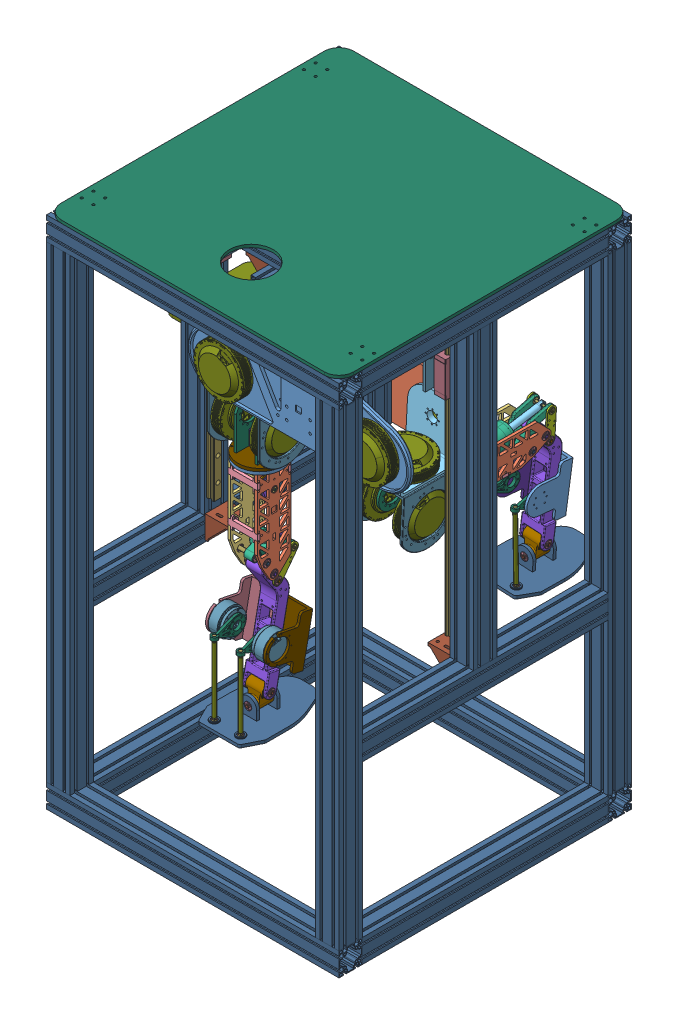
SolidWorks assembly 完整下肢, configuration 默认. Lengths in mm.
Overall size (1520 1770 1220).
259 component instances, 52 part files, 501 mates.
Components (placement in the parent):
- 髋一级连接板-1: 髋一级连接板 [默认] at (-1.8233 -129.1825 751.7525) size (760.75 280 18)
- 髋一级连接板_B-1: 髋一级连接板_B [默认] at (-1.8233 -129.1825 543.7525) size (760.75 280 18)
- 轴承_NSK635-1: 轴承_NSK635 [默认] at (238.0767 -238.3366 462.2655) x (0.049258 0.922114 0.38377) z (-0.020471 -0.383224 0.923429) size (19 6 19)
- 轴承_NSK635-2: 轴承_NSK635 [默认] at (-250.8233 -423.6825 652.2525) x (0 0.998125 -0.061201) z (0 0.061201 0.998125) size (19 6 19)
- 轴承_NSK635-3: 轴承_NSK635 [默认] at (142.2133 -233.2156 462.2655) x (0.049258 0.922114 0.38377) z (-0.020471 -0.383224 0.923429) size (19 6 19)
- 轴承_NSK635-4: 轴承_NSK635 [默认] at (-346.8233 -423.6825 652.2525) x (0 0.998125 -0.061201) z (0 0.061201 0.998125) size (19 6 19)
- 轴承_NSK6900NR-5: 轴承_NSK6900NR [默认] at (230.6224 -265.3994 255.8742) x (0.026574 0.497465 -0.867077) z (-0.046252 -0.865843 -0.498174) size (25 6 25)
- 轴承_NSK6900NR-6: 轴承_NSK6900NR [默认] at (231.9288 -240.9437 212.2827) x (0.026574 0.497465 -0.867077) z (-0.046252 -0.865843 -0.498174) size (25 6 25)
- 轴承_NSK6900NR-7: 轴承_NSK6900NR [默认] at (-256.8233 -630.3812 677.2525) x (0 0.205526 -0.978652) z (0 -0.978652 -0.205526) size (25 6 25)
- 轴承_NSK6900NR-8: 轴承_NSK6900NR [默认] at (140.7506 -260.5986 255.8742) x (0.049258 0.922114 0.38377) z (-0.020471 -0.383224 0.923429) size (25 6 25)
- 轴承_NSK6900NR-9: 轴承_NSK6900NR [默认] at (-256.8233 -673.6825 652.2525) x (0 0.205526 -0.978652) z (0 -0.978652 -0.205526) size (25 6 25)
- 轴承_NSK6900NR-10: 轴承_NSK6900NR [默认] at (-346.8233 -630.3812 677.2525) x (0 0.998125 -0.061201) z (0 0.061201 0.998125) size (25 6 25)
- 轴承_NSK6900NR-11: 轴承_NSK6900NR [默认] at (142.057 -236.1429 212.2827) x (0.049258 0.922114 0.38377) z (-0.020471 -0.383224 0.923429) size (25 6 25)
- 轴承_NSK6900NR-12: 轴承_NSK6900NR [默认] at (-346.8233 -673.6825 652.2525) x (0 0.998125 -0.061201) z (0 0.061201 0.998125) size (25 6 25)
- 轴承_NSK6900NR-17: 轴承_NSK6900NR [默认] at (176.6993 -262.5189 255.8742) x (0.000691 0.01293 0.999916) z (-0.053338 -0.998493 0.012949) size (25 6 25)
- 轴承_NSK6900NR-18: 轴承_NSK6900NR [默认] at (194.6737 -263.4791 255.8742) x (-0.021069 -0.394415 -0.918691) z (-0.049005 -0.917383 0.394978) size (25 6 25)
- 轴承_NSK6900NR-19: 轴承_NSK6900NR [默认] at (-310.8233 -630.3812 677.2525) x (0 -0.990009 -0.141004) z (0 0.141004 -0.990009) size (25 6 25)
- 轴承_NSK6900NR-20: 轴承_NSK6900NR [默认] at (-292.8233 -630.3812 677.2525) x (0 0.96851 -0.248973) z (0 -0.248973 -0.96851) size (25 6 25)
- 轴承_NSK6900NR-37: 轴承_NSK6900NR [默认] at (-324.8233 -1030.6139 652.2525) x (0 -0.237164 0.97147) z (0 -0.97147 -0.237164) size (25 6 25)
- 轴承_NSK6900NR-38: 轴承_NSK6900NR [默认] at (-278.8233 -1030.6139 652.2525) x (0 -0.153045 -0.988219) z (0 -0.988219 0.153045) size (25 6 25)
- 轴承_NSK6900NR-39: 轴承_NSK6900NR [默认] at (-301.8233 -1070.6139 629.2525) x (0.998149 0.060814 0) z (-0.060814 0.998149 0) size (25 6 25)
- 轴承_NSK6900NR-40: 轴承_NSK6900NR [默认] at (-301.8233 -1070.6139 675.2525) x (-0.802358 -0.596843 0) z (-0.596843 0.802358 0) size (25 6 25)
- 轴承_NSK6900NR-41: 轴承_NSK6900NR [默认] at (165.9394 -632.6645 198.3743) x (0.811883 -0.583783 0.006592) z (-0.58382 -0.811818 0.010283) size (25 6 25)
- 轴承_NSK6900NR-42: 轴承_NSK6900NR [默认] at (191.0252 -594.2319 174.8875) x (0.018298 0.342539 0.939325) z (0.050106 0.937988 -0.343027) size (25 6 25)
- 轴承_NSK6900NR-43: 轴承_NSK6900NR [默认] at (145.0907 -591.7781 174.8875) x (-0.004431 -0.082951 0.996544) z (-0.053158 -0.995125 -0.083069) size (25 6 25)
- 轴承_NSK6900NR-44: 轴承_NSK6900NR [默认] at (165.9094 -633.2256 152.3778) x (-0.360366 0.932744 -0.011143) z (-0.932811 -0.360332 0.005003) size (25 6 25)
- 轴承_NSK6900NR-45: 轴承_NSK6900NR [默认] at (-301.8233 -1070.6139 687.2525) x (-0.919919 -0.392109 0) z (-0.392109 0.919919 0) size (25 6 25)
- 轴承_NSK6900NR-46: 轴承_NSK6900NR [默认] at (-301.8233 -1070.6139 617.2525) x (0.999952 0.009828 0) z (-0.009828 0.999952 0) size (25 6 25)
- 轴承_NSK6900NR-47: 轴承_NSK6900NR [默认] at (165.9472 -632.5182 210.3734) x (-0.999254 0.038618 0.00018) z (0.038613 0.99918 -0.012213) size (25 6 25)
- 轴承_NSK6900NR-48: 轴承_NSK6900NR [默认] at (165.9016 -633.3719 140.3787) x (0.908248 -0.418407 0.004512) z (0.418431 0.908178 -0.01135) size (25 6 25)
- 轴承_NSK6900NR-33: 轴承_NSK6900NR [默认] at (-336.8233 -1030.6139 652.2525) x (0 -0.947209 0.320618) z (0 -0.320618 -0.947209) size (25 6 25)
- 轴承_NSK6900NR-34: 轴承_NSK6900NR [默认] at (203.0082 -594.872 174.8875) x (-0.049795 -0.932169 0.358581) z (0.019128 0.358071 0.933498) size (25 6 25)
- 轴承_NSK6900NR-35: 轴承_NSK6900NR [默认] at (-266.8233 -1030.6139 652.2525) x (0 -0.998208 -0.059843) z (0 -0.059843 0.998208) size (25 6 25)
- 轴承_NSK6900NR-36: 轴承_NSK6900NR [默认] at (133.1078 -591.138 174.8875) x (-0.053286 -0.997519 -0.046007) z (0.002454 0.045942 -0.998941) size (25 6 25)
- 轴承_NSK635-6: 轴承_NSK635 [默认] at (-275.8233 -643.2766 570.5287) x (0 0.998125 -0.061201) z (0 0.061201 0.998125) size (19 6 19)
- 轴承_NSK635-7: 轴承_NSK635 [默认] at (215.7047 -188.4726 179.8677) x (0.049258 0.922114 0.38377) z (-0.020471 -0.383224 0.923429) size (19 6 19)
- 轴承_NSK635-8: 轴承_NSK635 [默认] at (-321.8233 -643.2766 570.5287) x (0 0.998125 -0.061201) z (0 0.061201 0.998125) size (19 6 19)
- 轴承_NSK635-9: 轴承_NSK635 [默认] at (169.7702 -186.0189 179.8677) x (0.049258 0.922114 0.38377) z (-0.020471 -0.383224 0.923429) size (19 6 19)
- 轴承_NSK6900NR-21: 轴承_NSK6900NR [默认] at (215.8968 -278.61 180.3417) x (0.026574 0.497465 -0.867077) z (-0.046252 -0.865843 -0.498174) size (25 6 25)
- 轴承_NSK6900NR-22: 轴承_NSK6900NR [默认] at (153.9851 -275.3027 180.3417) x (0.047078 0.8813 0.470205) z (-0.025082 -0.469536 0.882557) size (25 6 25)
- 轴承_NSK6900NR-23: 轴承_NSK6900NR [默认] at (-332.8233 -715.285 624.5175) x (0 0.998125 -0.061201) z (0 0.061201 0.998125) size (25 6 25)
- 轴承_NSK6900NR-24: 轴承_NSK6900NR [默认] at (-270.8233 -715.285 624.5175) x (0 0.205526 -0.978652) z (0 -0.978652 -0.205526) size (25 6 25)
- 轴承_NSK6900NR-25: 轴承_NSK6900NR [默认] at (163.0271 -237.2631 212.2827) x (-0.000432 -0.00809 0.999967) z (-0.053341 -0.998543 -0.008101) size (25 6 25)
- 轴承_NSK6900NR-26: 轴承_NSK6900NR [默认] at (210.9587 -239.8235 212.2827) x (-0.022004 -0.411917 -0.910956) z (-0.048593 -0.909659 0.412504) size (25 6 25)
- 轴承_NSK6900NR-27: 轴承_NSK6900NR [默认] at (160.9751 -275.6761 180.3417) x (-0.000432 -0.00809 0.999967) z (-0.053341 -0.998543 -0.008101) size (25 6 25)
- 轴承_NSK6900NR-28: 轴承_NSK6900NR [默认] at (208.9068 -278.2366 180.3417) x (-0.000432 -0.00809 0.999967) z (0.053341 0.998543 0.008101) size (25 6 25)
- 轴承_NSK6900NR-29: 轴承_NSK6900NR [默认] at (-325.8233 -673.6825 652.2525) x (0 -0.98581 -0.167864) z (0 0.167864 -0.98581) size (25 6 25)
- 轴承_NSK6900NR-30: 轴承_NSK6900NR [默认] at (-277.8233 -715.285 624.5175) x (0 -0.98581 -0.167864) z (0 -0.167864 0.98581) size (25 6 25)
- 轴承_NSK6900NR-31: 轴承_NSK6900NR [默认] at (-325.8233 -715.285 624.5175) x (0 0.974921 -0.222553) z (0 0.222553 0.974921) size (25 6 25)
- 轴承_NSK6900NR-32: 轴承_NSK6900NR [默认] at (-277.8233 -673.6825 652.2525) x (0 0.974921 -0.222553) z (0 -0.222553 -0.974921) size (25 6 25)
- 轴承_NSK635-10: 轴承_NSK635 [默认] at (-270.8233 -643.2766 570.5287) x (0 0.138285 -0.990392) z (0 -0.990392 -0.138285) size (19 6 19)
- 轴承_NSK635-11: 轴承_NSK635 [默认] at (158.7858 -185.4321 179.8677) x (0.000691 0.01293 0.999916) z (-0.053338 -0.998493 0.012949) size (19 6 19)
- 轴承_NSK635-12: 轴承_NSK635 [默认] at (-338.8233 -643.2766 570.5287) x (0 0.091476 -0.995807) z (0 -0.995807 -0.091476) size (19 6 19)
- 轴承_NSK635-13: 轴承_NSK635 [默认] at (226.689 -189.0594 179.8677) x (0.000691 0.01293 0.999916) z (-0.053338 -0.998493 0.012949) size (19 6 19)
- 髋二级连接板_旋转-1: 髋二级连接板_旋转 [默认] at (-216.8233 -124.1825 562.2525) x (0 0 -1) z (-1 0 0) size (206.5 183 170)
- 髋二级连接板_旋转-2: 髋二级连接板_旋转 [默认] at (277.9881 -128.5814 562.2525) x (0 0 -1) z (-0.998576 0.053343 0) size (206.5 183 170)
- 大腿_电机轴-1: 大腿_电机轴 [默认] at (241.0724 -238.4966 462.2655) x (0.049258 0.922114 0.38377) z (-0.020471 -0.383224 0.923429) size (5 108 5)
- 大腿_电机轴-2: 大腿_电机轴 [默认] at (-247.8233 -423.6825 652.2525) x (0 -0.967053 0.254576) z (0 -0.254576 -0.967053) size (5 108 5)
- 上下连杆轴-1: 上下连杆轴 [默认] at (229.6848 -189.2194 179.8677) x (-0.049961 -0.935279 -0.350368) z (-0.998576 0.053343 0) size (5 5 80)
- 上下连杆轴-2: 上下连杆轴 [默认] at (-341.8233 -643.2766 570.5287) x (0 0.004287 -0.999991) z (1 0 0) size (5 5 80)
- 大腿小腿轴-1: 大腿小腿轴 [默认] at (186.9929 -238.5433 212.2827) x (0.050119 0.93823 0.342364) z (-0.018263 -0.341876 0.939568) size (10 108 10)
- 大腿小腿轴-2: 大腿小腿轴 [默认] at (-301.8233 -673.6825 652.2525) x (0 0.99823 -0.059474) z (0 0.059474 0.99823) size (10 108 10)
- 下连杆小腿轴-1: 下连杆小腿轴 [默认] at (184.9409 -276.9563 180.3417) x (0.049345 0.923729 0.379855) z (-0.020263 -0.379314 0.925046) size (10 80 10)
- 下连杆小腿轴-2: 下连杆小腿轴 [默认] at (-301.8233 -715.285 624.5175) x (0 0.99823 -0.059474) z (0 0.059474 0.99823) size (10 80 10)
- 上连杆大腿轴-1: 上连杆大腿轴 [默认] at (-301.8233 -630.3812 677.2525) x (0 0.998125 -0.061201) z (0 0.061201 0.998125) size (10 108 10)
- 上连杆大腿轴-2: 上连杆大腿轴 [默认] at (185.6865 -262.999 255.8742) x (0.049258 0.922114 0.38377) z (-0.020471 -0.383224 0.923429) size (10 108 10)
- 踝关节轴-3: 踝关节轴 [默认] at (-301.8233 -1070.6139 652.2525) x (0.999952 0.009828 0) z (-0.009828 0.999952 0) size (10 88 10)
- 踝关节轴-4: 踝关节轴 [默认] at (165.9244 -632.945 175.376) x (0.908248 -0.418407 0.004512) z (0.418431 0.908178 -0.01135) size (10 88 10)
- 踝关节轴-1: 踝关节轴 [默认] at (168.058 -593.005 174.8875) x (-0.048986 -0.917023 0.395815) z (0.021114 0.395252 0.91833) size (10 88 10)
- 踝关节轴-2: 踝关节轴 [默认] at (-301.8233 -1030.6139 652.2525) x (0 -0.998208 -0.059843) z (0 -0.059843 0.998208) size (10 88 10)
- 轴套-3: 轴套 [d5L40.5大腿板与电机] at (182.6557 -235.376 462.2655) x (0.000691 0.01293 0.999916) z (-0.998576 0.053343 0) size (7 7 40.5)
- 轴套-4: 轴套 [d5L40.5大腿板与电机] at (232.0852 -238.0165 462.2655) x (0.000691 0.01293 0.999916) z (-0.998576 0.053343 0) size (7 7 40.5)
- 轴套-5: 轴套 [d5L40.5大腿板与电机] at (-297.3233 -423.6825 652.2525) x (0 0.004287 -0.999991) z (1 0 0) size (7 7 40.5)
- 轴套-6: 轴套 [d5L40.5大腿板与电机] at (-346.8233 -423.6825 652.2525) x (0 0.004287 -0.999991) z (1 0 0) size (7 7 40.5)
- 轴套-11: 轴套 [d5L5上下连杆] at (-332.8233 -643.2766 570.5287) x (0 0.259292 -0.965799) z (1 0 0) size (7 7 5)
- 轴套-12: 轴套 [d5L5上下连杆] at (163.7787 -185.6988 179.8677) x (0.000691 0.01293 0.999916) z (-0.998576 0.053343 0) size (7 7 5)
- 轴套-13: 轴套 [d5L5上下连杆] at (-275.8233 -643.2766 570.5287) x (0 0.004287 -0.999991) z (1 0 0) size (7 7 5)
- 轴套-14: 轴套 [d5L5上下连杆] at (220.6976 -188.7394 179.8677) x (0.000691 0.01293 0.999916) z (-0.998576 0.053343 0) size (7 7 5)
- 轴套-15: 轴套 [d5L15.5上连杆与推杆] at (209.7132 -188.1526 179.8677) x (0.000691 0.01293 0.999916) z (-0.998576 0.053343 0) size (7 7 15.5)
- 轴套-16: 轴套 [d5L15.5上连杆与推杆] at (185.2481 -186.8457 179.8677) x (0.007725 0.144605 0.989459) z (-0.998576 0.053343 0) size (7 7 15.5)
- 轴套-17: 轴套 [d5L15.5上连杆与推杆] at (-297.3233 -643.2766 570.5287) x (0 0.004287 -0.999991) z (1 0 0) size (7 7 15.5)
- 轴套-18: 轴套 [d5L15.5上连杆与推杆] at (-321.8233 -643.2766 570.5287) x (0 0.004287 -0.999991) z (1 0 0) size (7 7 15.5)
- 轴套-19: 轴套 [d10L15大小腿] at (231.9288 -240.9437 212.2827) x (0.00702 0.131424 0.991301) z (-0.998576 0.053343 0) size (12 12 15)
- 轴套-20: 轴套 [d10L15大小腿] at (-346.8233 -673.6825 652.2525) x (0 0.00111 -0.999999) z (1 0 0) size (12 12 15)
- 轴套-21: 轴套 [d10L15大小腿] at (157.0356 -236.943 212.2827) x (-0.000432 -0.00809 0.999967) z (-0.998576 0.053343 0) size (12 12 15)
- 轴套-22: 轴套 [d10L15大小腿] at (-271.8233 -673.6825 652.2525) x (0 -0.961131 -0.276091) z (1 0 0) size (12 12 15)
- 轴套-23: 轴套 [d10L1小腿下连杆] at (-331.8233 -715.285 624.5175) x (0 0.98581 0.167864) z (-1 0 0) size (12 12 1)
- 轴套-24: 轴套 [d10L1小腿下连杆] at (153.9851 -275.3027 180.3417) x (-0.029978 -0.561194 -0.827141) z (0.998576 -0.053343 0) size (12 12 1)
- 轴套-25: 轴套 [d10L1小腿下连杆] at (-271.8233 -715.285 624.5175) x (0 0.011403 -0.999935) z (1 0 0) size (12 12 1)
- 轴套-26: 轴套 [d10L1小腿下连杆] at (215.8968 -278.61 180.3417) x (-0.000432 -0.00809 0.999967) z (-0.998576 0.053343 0) size (12 12 1)
- 轴套-7: 轴套 [d10L30大腿上连杆] at (170.7079 -262.1989 255.8742) x (-0.024462 -0.457931 0.888651) z (-0.998576 0.053343 0) size (12 12 30)
- 轴套-8: 轴套 [d10L30大腿上连杆] at (230.6224 -265.3994 255.8742) x (0.001085 0.020314 0.999793) z (-0.998576 0.053343 0) size (12 12 30)
- 轴套-9: 轴套 [d10L30大腿上连杆] at (-286.8233 -630.3812 677.2525) x (0 0.004287 -0.999991) z (1 0 0) size (12 12 30)
- 轴套-10: 轴套 [d10L30大腿上连杆] at (-346.8233 -630.3812 677.2525) x (0 -0.022464 -0.999748) z (1 0 0) size (12 12 30)
- 轴套V2-1: 轴套V2 [d10L6踝关节] at (-272.8233 -1030.6139 652.2525) x (0 0.885448 0.464738) z (1 0 0) size (12 12 6)
- 轴套V2-2: 轴套V2 [d10L6踝关节] at (-336.8233 -1030.6139 652.2525) x (0 -0.178991 -0.983851) z (1 0 0) size (12 12 6)
- 轴套V2-3: 轴套V2 [d10L6踝关节] at (139.0993 -591.458 174.8875) x (-0.003743 -0.070062 0.997536) z (-0.998576 0.053343 0) size (12 12 6)
- 轴套V2-4: 轴套V2 [d10L6踝关节] at (203.0082 -594.872 174.8875) x (-0.012193 -0.228259 0.973524) z (-0.998576 0.053343 0) size (12 12 6)
- 轴套-27: 轴套 [d10L6踝关节] at (-301.8233 -1070.6139 681.2525) x (0.999952 0.009828 0) z (0 0 1) size (12 12 6)
- 轴套-28: 轴套 [d10L6踝关节] at (-301.8233 -1070.6139 617.2525) x (0.999952 0.009828 0) z (0 0 1) size (12 12 6)
- 轴套-29: 轴套 [d10L6踝关节] at (165.9016 -633.3719 140.3787) x (0.908248 -0.418407 0.004512) z (0.000652 0.012197 0.999925) size (12 12 6)
- 轴套-30: 轴套 [d10L6踝关节] at (165.9433 -632.5913 204.3739) x (0.908248 -0.418407 0.004512) z (0.000652 0.012197 0.999925) size (12 12 6)
- 髋三级连接板_前摆V2-1: 髋三级连接板_前摆V2 [默认] at (181.9338 -333.249 562.2525) x (0.998576 -0.053343 0) z (0 0 1) size (180 200 180)
- 髋三级连接板_前摆V2-2: 髋三级连接板_前摆V2 [默认] at (-301.8233 -333.6825 742.2525) x (-1 0 0) z (0 0 -1) size (180 200 180)
- 腿髋转接架侧板V2-1: 腿髋转接架侧板V2 [默认] at (227.1486 -236.696 552.2594) x (-0.053339 -0.998508 0.011726) z (-0.998576 0.053343 0) size (96 150 8)
- 腿髋转接架侧板V2-2: 腿髋转接架侧板V2 [默认] at (147.2625 -232.4286 552.2594) x (0.053339 0.998508 -0.011726) z (0.998576 -0.053343 0) size (96 150 8)
- 腿髋转接架侧板V2-3: 腿髋转接架侧板V2 [默认] at (-261.8233 -333.6825 652.2525) x (0 0 1) z (-1 0 0) size (96 150 8)
- 腿髋转接架侧板V2-4: 腿髋转接架侧板V2 [默认] at (-341.8233 -333.6825 652.2525) x (0 0 -1) z (1 0 0) size (96 150 8)
- B1电机模型-1: B1电机模型 [默认] at (349.6629 49.3918 700.037) x (0 0 1) z (-0.906308 -0.422618 0) size (57.67 170.5 170.5)
- B1电机模型-2: B1电机模型 [默认] at (181.2585 -154.384 500.7663) x (0.998576 -0.053343 0) z (-0.022544 -0.422017 0.906308) size (57.67 170.5 170.5)
- B1电机模型-3: B1电机模型 [默认] at (193.9731 -299.3815 809.8173) x (-0.998576 0.053343 0) z (0.022544 0.422017 -0.906308) size (57.67 170.5 170.5)
- B1电机模型-4: B1电机模型 [默认] at (-144.2585 -94.7211 700.037) x (0 0 1) z (-0.906308 0.422618 0) size (57.67 170.5 170.5)
- B1电机模型-6: B1电机模型 [默认] at (124.4785 -180.1818 809.8173) x (0.053343 0.998576 0) z (0.422017 -0.022544 -0.906308) size (57.67 170.5 170.5)
- B1电机模型-7: B1电机模型 [默认] at (-380.3976 -183.898 500.7663) x (0 1 0) z (0.422618 0 0.906308) size (57.67 170.5 170.5)
- B1电机模型-10: B1电机模型 [默认] at (-291.6078 -299.2211 809.8173) x (-1 0 0) z (0 0.422618 -0.906308) size (57.67 170.5 170.5)
- B1电机模型-11: B1电机模型 [默认] at (-312.0388 -155.1082 500.7663) x (1 0 0) z (0 -0.422618 0.906308) size (57.67 170.5 170.5)
- 腿髋转接架连接板V2-1: 腿髋转接架连接板V2 [默认] at (-333.8233 -333.6825 647.2525) size (30 50 10)
- 腿髋转接架连接板V2-2: 腿髋转接架连接板V2 [默认] at (218.8933 -241.2618 552.318) x (-0.998576 0.053343 0) z (0.053339 0.998508 -0.011726) size (30 50 10)
- 腿髋转接架连接板V2-3: 腿髋转接架连接板V2 [默认] at (155.5178 -227.8628 552.2007) x (0.998576 -0.053343 0) z (-0.053339 -0.998508 0.011726) size (30 50 10)
- 腿髋转接架连接板V2-4: 腿髋转接架连接板V2 [默认] at (-269.8233 -333.6825 657.2525) x (-1 0 0) z (0 0 -1) size (30 50 10)
- 腿髋转接架底座V2-1: 腿髋转接架底座V2 [默认] at (187.2056 -234.5623 552.2594) x (-0.998576 0.053343 0) z (-0.053339 -0.998508 0.011726) size (150 10 150)
- 腿髋转接架底座V2-2: 腿髋转接架底座V2 [默认] at (-301.8233 -333.6825 652.2525) x (-1 0 0) z (0 0 1) size (150 10 150)
- 大腿主干_上板V2-1: 大腿主干_上板V2 [默认] at (-301.8233 -673.6825 602.2525) size (150 10 150)
- 大腿主干_上板V2-2: 大腿主干_上板V2 [默认] at (189.6599 -188.6179 211.6964) x (0.998576 -0.053343 0) z (-0.053339 -0.998508 0.011726) size (150 10 150)
- 大腿主干_右侧板V2-1: 大腿主干_右侧板V2 [默认] at (236.9217 -241.2105 212.2827) x (-0.053339 -0.998508 0.011726) z (-0.998576 0.053343 0) size (116 518 200.95)
- 大腿主干_右侧板V2-2: 大腿主干_右侧板V2 [默认] at (-251.8233 -673.6825 652.2525) x (0 0 1) z (-1 0 0) size (116 518 200.95)
- 大腿主干_左侧板V2-1: 大腿主干_左侧板V2 [默认] at (236.9217 -241.2105 212.2827) x (-0.053339 -0.998508 0.011726) z (-0.998576 0.053343 0) size (116 518 200.95)
- 大腿主干_左侧板V2-2: 大腿主干_左侧板V2 [默认] at (-251.8233 -673.6825 652.2525) x (0 0 1) z (-1 0 0) size (116 518 200.95)
- 大腿侧板连接V2-1: 大腿侧板连接V2 [默认] at (233.9061 -297.6638 337.6571) x (0.000625 0.011709 0.999931) z (-0.998576 0.053343 0) size (40 20 100)
- 大腿侧板连接V2-2: 大腿侧板连接V2 [默认] at (-351.8233 -398.6825 594.2525) x (0 1 0) z (1 0 0) size (40 20 100)
- 大腿侧板连接V2-3: 大腿侧板连接V2 [默认] at (-251.8233 -548.9797 710.2525) x (0 1 0) z (-1 0 0) size (40 20 100)
- 大腿侧板连接V2-4: 大腿侧板连接V2 [默认] at (234.0001 -295.9039 487.9439) x (0.000625 0.011709 0.999931) z (-0.998576 0.053343 0) size (40 20 100)
- 大腿侧板连接V2-5: 大腿侧板连接V2 [默认] at (240.1999 -179.8429 506.5824) x (-0.000625 -0.011709 -0.999931) z (-0.998576 0.053343 0) size (40 20 100)
- 大腿侧板连接V2-6: 大腿侧板连接V2 [默认] at (-251.8233 -398.6825 710.2525) x (0 1 0) z (-1 0 0) size (40 20 100)
- 大腿主干_连接块-1: 大腿主干_连接块 [默认] at (228.4014 -231.991 532.2021) x (-0.998576 0.053343 0) z (-0.053339 -0.998508 0.011726) size (40 50 10)
- 大腿主干_连接块-2: 大腿主干_连接块 [默认] at (145.9847 -237.6019 532.3194) x (0.998576 -0.053343 0) z (0.053339 0.998508 -0.011726) size (40 50 10)
- 大腿主干_连接块-3: 大腿主干_连接块 [默认] at (-342.8233 -353.6825 657.2525) x (1 0 0) z (0 0 -1) size (40 50 10)
- 大腿主干_连接块-4: 大腿主干_连接块 [默认] at (-260.8233 -353.6825 647.2525) x (-1 0 0) z (0 0 1) size (40 50 10)
- 膝盖上连杆_107.5V2-1: 膝盖上连杆_107.5V2 [默认] at (224.6919 -188.9527 179.8677) x (-0.051524 -0.964525 -0.258915) z (-0.998576 0.053343 0) size (83.75 123.1 70)
- 膝盖上连杆_107.5V2-2: 膝盖上连杆_107.5V2 [默认] at (-266.8233 -643.2766 570.5287) x (0 -0.799794 0.600275) z (-1 0 0) size (83.75 123.1 70)
- 膝关节下连杆_90-1: 膝关节下连杆_90 [默认] at (220.8897 -278.8767 180.3417) x (0.000281 0.005259 0.999986) z (-0.998576 0.053343 0) size (30 120 76)
- 膝关节下连杆_90-2: 膝关节下连杆_90 [默认] at (-337.8233 -715.285 624.5175) x (0 -0.599875 -0.800094) z (1 0 0) size (30 120 76)
- 小腿主干-1: 小腿主干 [默认] at (216.9502 -240.1436 212.2827) x (0.004924 0.092171 0.995731) z (-0.998576 0.053343 0) size (110 390 143.66)
- 小腿主干-2: 小腿主干 [默认] at (-271.8233 -673.6825 652.2525) x (0 0.196116 0.980581) z (-1 0 0) size (110 390 143.66)
- 脚踝十字连接-1: 脚踝十字连接 [默认] at (-330.8233 -1030.6139 652.2525) x (0 -1 0) z (1 0 0) size (80 58 58)
- 脚踝十字连接-2: 脚踝十字连接 [默认] at (197.0167 -594.5519 174.8875) x (-0.053339 -0.998502 0.012214) z (-0.998576 0.053343 0) size (80 58 58)
- 球铰脚底板-1: 球铰脚底板 [默认] at (-301.8233 -1110.6139 792.2525) size (200 93.12 300)
- 球铰脚底板-2: 球铰脚底板 [默认] at (163.8821 -671.1776 315.8542) x (0.998576 -0.053343 0) z (0.000652 0.012197 0.999925) size (200 93.12 300)
- 关节轴承外圈_SQD6-1: 关节轴承外圈_SQD6 [默认] at (209.1919 -666.5799 285.7663) x (-0.053339 -0.998502 0.012214) z (0.009299 0.011734 0.999888) size (6.75 18 18)
- 关节轴承外圈_SQD6-2: 关节轴承外圈_SQD6 [默认] at (119.32 -661.7791 285.7663) x (-0.053339 -0.998502 0.012214) z (0.009299 0.011734 0.999888) size (6.75 18 18)
- 关节轴承外圈_SQD6-3: 关节轴承外圈_SQD6 [默认] at (-256.8233 -1103.2389 762.2525) x (0 -1 0) z (-0.68418 0 0.729313) size (6.75 18 18)
- 关节轴承外圈_SQD6-4: 关节轴承外圈_SQD6 [默认] at (-346.8233 -1103.2389 762.2525) x (0 -1 0) z (-0.68418 0 0.729313) size (6.75 18 18)
- 关节轴承内杆_SQD6-1: 关节轴承内杆_SQD6 [默认] at (-346.8233 -1103.2389 762.2525) x (0.998471 0 -0.055281) z (0.055281 0.000001 0.998471) size (14 37.17 14)
- 关节轴承内杆_SQD6-2: 关节轴承内杆_SQD6 [默认] at (-256.8233 -1103.2389 762.2525) x (0.998075 0 -0.062014) z (0.062014 0.000001 0.998075) size (14 37.17 14)
- 关节轴承内杆_SQD6-3: 关节轴承内杆_SQD6 [默认] at (119.32 -661.7791 285.7663) x (0.707856 -0.086337 0.70106) z (-0.704349 -0.011501 0.70976) size (14 37.17 14)
- 关节轴承内杆_SQD6-4: 关节轴承内杆_SQD6 [默认] at (209.1919 -666.5799 285.7663) x (0.998399 -0.051754 -0.02282) z (0.019165 -0.070057 0.997359) size (14 37.17 14)
- 小腿左侧电机安装板A1-1: 小腿左侧电机安装板A1 [默认] at (-404.8233 -957.0654 606.9487) x (1 0 0) z (0 0.196116 0.980581) size (99.5 170 146)
- A1电机-1: A1电机 [默认] at (-395.8233 -854.1044 688.3369) x (0 0.194064 -0.980989) z (1 0 0) size (92 92 49)
- 小腿电机摇杆A1-1: 小腿电机摇杆A1 [默认] at (-343.8233 -854.1044 688.3369) x (0 0.002916 0.999996) z (-1 0 0) size (114.92 60 22)
- 关节轴承外圈_SQD6-5: 关节轴承外圈_SQD6 [默认] at (-346.8233 -853.8889 762.2522) x (0 -0.999996 0.002916) z (0.078101 0.002907 0.996941) size (6.75 18 18)
- 关节轴承内杆_SQD6-5: 关节轴承内杆_SQD6 [默认] at (-346.8233 -853.8889 762.2522) x (-0.959854 0 -0.280502) z (-0.280502 0.000001 0.959854) size (14 37.17 14)
- 踝关节连杆-1: 踝关节连杆 [默认] at (-346.8233 -1091.0639 762.2525) x (0.267051 -0.000001 -0.963682) z (0 1 -0.000001) size (12 12 225)
- 小腿左侧定脚踝安装板-1: 小腿左侧定脚踝安装板 [默认] at (114.2954 -512.1318 137.5386) x (0.998576 -0.053343 0) z (0.004924 0.092171 0.995731) size (54.5 170 146)
- 小腿电机摇杆A1-3: 小腿电机摇杆A1 [默认] at (135.2798 -419.2516 229.2659) x (0.00413 0.077315 0.996998) z (-0.998576 0.053343 0) size (114.92 60 22)
- 关节轴承内杆_SQD6-6: 关节轴承内杆_SQD6 [默认] at (132.5894 -413.3767 302.9597) x (0.23447 -0.079585 0.96886) z (0.970666 -0.035391 -0.237814) size (14 37.17 14)
- 关节轴承外圈_SQD6-6: 关节轴承外圈_SQD6 [默认] at (132.5894 -413.3767 302.9597) x (0.053183 0.995579 -0.077426) z (-0.981979 0.066222 0.177009) size (6.75 18 18)
- 踝关节连杆-2: 踝关节连杆 [默认] at (131.9415 -425.5054 302.1202) x (-0.140449 -0.060897 0.988213) z (-0.053216 -0.9962 -0.068953) size (12 12 225)
- 镜向小腿左侧电机安装板A1-3: 镜向小腿左侧电机安装板A1 [默认] at (-198.8233 -957.0654 606.9487) x (-1 0 0) z (0 -0.196116 -0.980581) size (99.5 170 146)
- 镜向小腿左侧定脚踝安装板-2: 镜向小腿左侧定脚踝安装板 [默认] at (230.1303 -518.3196 137.5386) x (-0.998576 0.053343 0) z (-0.004924 -0.092171 -0.995731) size (54.5 170 146)
- 小腿电机摇杆A1-4: 小腿电机摇杆A1 [默认] at (225.1517 -424.0524 229.2659) x (0.00413 0.077315 0.996998) z (-0.998576 0.053343 0) size (114.92 60 22)
- 关节轴承内杆_SQD6-8: 关节轴承内杆_SQD6 [默认] at (222.4612 -418.1776 302.9597) x (0.994388 -0.059188 0.087687) z (0.091435 0.063899 -0.993759) size (14 37.17 14)
- 关节轴承外圈_SQD6-8: 关节轴承外圈_SQD6 [默认] at (222.4612 -418.1776 302.9597) x (0.053183 0.995579 -0.077426) z (-0.112914 0.083033 0.990129) size (6.75 18 18)
- 踝关节连杆-4: 踝关节连杆 [默认] at (209.8398 -654.4512 286.6058) x (0.99813 -0.055144 0.026366) z (0.053216 0.9962 0.068953) size (12 12 225)
- 小腿电机摇杆A1-5: 小腿电机摇杆A1 [默认] at (-253.8233 -854.1044 688.3369) x (0 0.002916 0.999996) z (-1 0 0) size (114.92 60 22)
- A1电机-3: A1电机 [默认] at (-207.8233 -854.1044 688.3369) x (0 -0.194064 0.980989) z (-1 0 0) size (92 92 49)
- 关节轴承内杆_SQD6-9: 关节轴承内杆_SQD6 [默认] at (-256.8233 -853.8889 762.2522) x (0.971204 0 -0.238248) z (-0.238248 -0.000001 -0.971204) size (14 37.17 14)
- 关节轴承外圈_SQD6-9: 关节轴承外圈_SQD6 [默认] at (-256.8233 -853.8889 762.2522) x (0 -0.999996 0.002916) z (-0.243757 0.002828 0.969832) size (6.75 18 18)
- 踝关节连杆-5: 踝关节连杆 [默认] at (-256.8233 -866.0639 762.2522) x (0.999941 0 -0.010841) z (0 -1 0.000001) size (12 12 225)
- 轴用挡圈GB894-5-1: 轴用挡圈GB894-5 [默认] at (135.7226 -232.8689 462.2655) x (-0.050634 -0.947874 0.314595) z (0.016781 0.314148 0.949226) size (6.4 0.5 7.57)
- 轴用挡圈GB894-5-2: 轴用挡圈GB894-5 [默认] at (-352.8233 -423.6825 652.2525) x (0 0.998504 -0.054676) z (0 0.054676 0.998504) size (6.4 0.5 7.57)
- 轴用挡圈GB894-5-3: 轴用挡圈GB894-5 [默认] at (-250.3233 -423.6825 652.2525) x (0 0.998504 -0.054676) z (0 0.054676 0.998504) size (6.4 0.5 7.57)
- 轴用挡圈GB894-5-4: 轴用挡圈GB894-5 [默认] at (238.576 -238.3632 462.2655) x (-0.052938 -0.991004 0.122918) z (-0.006557 -0.122743 -0.992417) size (6.4 0.5 7.57)
- 轴用挡圈GB894-5-5: 轴用挡圈GB894-5 [默认] at (-264.3233 -643.2766 570.5287) x (0 0.998504 -0.054676) z (0 0.054676 0.998504) size (6.4 0.5 7.57)
- 轴用挡圈GB894-5-6: 轴用挡圈GB894-5 [默认] at (227.1883 -189.0861 179.8677) x (-0.052938 -0.991004 0.122918) z (-0.006557 -0.122743 -0.992417) size (6.4 0.5 7.57)
- 轴用挡圈GB894-5-7: 轴用挡圈GB894-5 [默认] at (152.2951 -185.0854 179.8677) x (-0.050634 -0.947874 0.314595) z (0.016781 0.314148 0.949226) size (6.4 0.5 7.57)
- 轴用挡圈GB894-5-8: 轴用挡圈GB894-5 [默认] at (-339.3233 -643.2766 570.5287) x (0 0.186477 -0.982459) z (0 -0.982459 -0.186477) size (6.4 0.5 7.57)
- 轴用挡圈GB894-10-5: 轴用挡圈GB894-10 [默认] at (-353.8233 -630.3812 677.2525) x (0 0.186477 -0.982459) z (0 -0.982459 -0.186477) size (11.5 1 12.44)
- 轴用挡圈GB894-10-6: 轴用挡圈GB894-10 [默认] at (-353.8233 -673.6825 652.2525) x (0 0.186477 -0.982459) z (0 -0.982459 -0.186477) size (11.5 1 12.44)
- 轴用挡圈GB894-10-7: 轴用挡圈GB894-10 [默认] at (-339.8233 -715.285 624.5175) x (0 0.186477 -0.982459) z (0 -0.982459 -0.186477) size (11.5 1 12.44)
- 轴用挡圈GB894-10-8: 轴用挡圈GB894-10 [默认] at (133.7605 -260.2252 255.8742) x (-0.050634 -0.947874 0.314595) z (0.016781 0.314148 0.949226) size (11.5 1 12.44)
- 轴用挡圈GB894-10-9: 轴用挡圈GB894-10 [默认] at (135.0669 -235.7695 212.2827) x (-0.050634 -0.947874 0.314595) z (0.016781 0.314148 0.949226) size (11.5 1 12.44)
- 轴用挡圈GB894-10-10: 轴用挡圈GB894-10 [默认] at (146.995 -274.9293 180.3417) x (-0.050634 -0.947874 0.314595) z (0.016781 0.314148 0.949226) size (11.5 1 12.44)
- 轴用挡圈GB894-10-11: 轴用挡圈GB894-10 [默认] at (237.6125 -265.7728 255.8742) x (-0.052938 -0.991004 0.122918) z (-0.006557 -0.122743 -0.992417) size (11.5 1 12.44)
- 轴用挡圈GB894-10-12: 轴用挡圈GB894-10 [默认] at (238.9189 -241.3171 212.2827) x (-0.052938 -0.991004 0.122918) z (-0.006557 -0.122743 -0.992417) size (11.5 1 12.44)
- 轴用挡圈GB894-10-13: 轴用挡圈GB894-10 [默认] at (222.8868 -278.9834 180.3417) x (-0.052938 -0.991004 0.122918) z (-0.006557 -0.122743 -0.992417) size (11.5 1 12.44)
- 轴用挡圈GB894-10-14: 轴用挡圈GB894-10 [默认] at (-249.8233 -630.3812 677.2525) x (0 0.998504 -0.054676) z (0 0.054676 0.998504) size (11.5 1 12.44)
- 轴用挡圈GB894-10-15: 轴用挡圈GB894-10 [默认] at (-249.8233 -673.6825 652.2525) x (0 0.998504 -0.054676) z (0 0.054676 0.998504) size (11.5 1 12.44)
- 轴用挡圈GB894-10-16: 轴用挡圈GB894-10 [默认] at (-263.8233 -715.285 624.5175) x (0 0.998504 -0.054676) z (0 0.054676 0.998504) size (11.5 1 12.44)
- 轴用挡圈GB894-10-17: 轴用挡圈GB894-10 [默认] at (-259.8233 -1030.6139 652.2525) x (0 0.998504 -0.054676) z (0 0.054676 0.998504) size (11.5 1 12.44)
- 轴用挡圈GB894-10-18: 轴用挡圈GB894-10 [默认] at (209.9982 -595.2454 174.8875) x (-0.052938 -0.991004 0.122918) z (-0.006557 -0.122743 -0.992417) size (11.5 1 12.44)
- 轴用挡圈GB894-10-19: 轴用挡圈GB894-10 [默认] at (126.1178 -590.7646 174.8875) x (-0.050634 -0.947874 0.314595) z (0.016781 0.314148 0.949226) size (11.5 1 12.44)
- 轴用挡圈GB894-10-20: 轴用挡圈GB894-10 [默认] at (-343.8233 -1030.6139 652.2525) x (0 0.186477 -0.982459) z (0 -0.982459 -0.186477) size (11.5 1 12.44)
- 轴用挡圈GB894-10-21: 轴用挡圈GB894-10 [默认] at (165.8971 -633.4573 133.3792) x (-0.980019 -0.198879 0.003064) z (-0.198901 0.979948 -0.011824) size (11.5 1 12.44)
- 轴用挡圈GB894-10-22: 轴用挡圈GB894-10 [默认] at (-301.8233 -1070.6139 610.2525) x (0.997979 0.063544 0) z (0.063544 -0.997979 0) size (11.5 1 12.44)
- 轴用挡圈GB894-10-23: 轴用挡圈GB894-10 [默认] at (-301.8233 -1070.6139 694.2525) x (-0.943455 -0.331502 0) z (0.331502 -0.943455 0) size (11.5 1 12.44)
- 轴用挡圈GB894-10-24: 轴用挡圈GB894-10 [默认] at (165.9518 -632.4328 217.3729) x (0.945813 0.324678 -0.004577) z (-0.32471 0.945746 -0.011324) size (11.5 1 12.44)
- 孔用挡圈GB893-18-1: 孔用挡圈GB893-18 [默认] at (209.4252 -662.2115 285.7129) x (-0.053339 -0.998502 0.012214) z (0.109153 0.006328 0.994005) size (1.02 17.46 19.5)
- 孔用挡圈GB893-18-2: 孔用挡圈GB893-18 [默认] at (119.5 -658.4091 285.7251) x (0.053339 0.998502 -0.012214) z (-0.562826 0.040165 0.825599) size (1.02 17.46 19.5)
- 孔用挡圈GB893-18-3: 孔用挡圈GB893-18 [默认] at (-256.8233 -1099.8639 762.2525) x (0 1 0) z (0.066439 0 0.997791) size (1.02 17.46 19.5)
- 孔用挡圈GB893-18-4: 孔用挡圈GB893-18 [默认] at (-346.8233 -1098.8639 762.2525) x (0 -1 0) z (-0.500498 0 0.865737) size (1.02 17.46 19.5)
- 膝关节SEA801-188移动端-1: 膝关节SEA801-188移动端 [默认] at (199.6201 -22.5449 276.165) x (0.009047 0.169361 -0.985513) z (-0.05257 -0.984109 -0.169603) size (183.01 20.01 20.01)
- 膝关节SEA801-188主体-2: 膝关节SEA801-188主体 [默认] at (198.7014 -39.7434 376.2431) x (0.009047 0.169361 -0.985513) z (-0.05257 -0.984109 -0.169603) size (181.51 65.01 65.01)
- 交叉滚子轴承GL_XRU3515UUCC0P5-1: 交叉滚子轴承GL_XRU3515UUCC0P5 [默认] at (198.1767 -29.1825 536.2525) x (0.707107 0.707107 0) z (0.707107 -0.707107 0) size (95 15 95)
- 交叉滚子轴承GL_XRU3515UUCC0P5-2: 交叉滚子轴承GL_XRU3515UUCC0P5 [默认] at (-301.8233 -29.1825 536.2525) x (0.707107 0.707107 0) z (0.707107 -0.707107 0) size (95 15 95)
- 膝关节直立固定棒-1: 膝关节直立固定棒 [默认] at (-297.3233 -642.181 565.6014) x (0 0.937202 0.348787) z (-1 0 0) size (235 40 9)
- 膝关节直立固定棒_盖-1: 膝关节直立固定棒_盖 [默认] at (-297.3233 -648.8998 568.436) x (0 0.348787 -0.937202) z (0 0.937202 0.348787) size (40 9 5)
- 膝关节直立固定棒_盖-2: 膝关节直立固定棒_盖 [默认] at (-297.3233 -418.0593 654.3452) x (0 -0.348787 0.937202) z (0 -0.937202 -0.348787) size (40 9 5)
- GS8080D型材-1: GS8080D型材 [400] at (-120.3733 70.8175 591.7525) x (1 0 0) z (0 -1 0) size (80 80 400)
- GS8080D型材-2: GS8080D型材 [400] at (8.1267 70.8175 711.7525) x (1 0 0) z (0 -1 0) size (80 80 400)
- GS8080D型材-3: GS8080D型材 [400] at (8.1267 70.8175 591.7525) x (1 0 0) z (0 1 0) size (80 80 400)
- GS8080D型材-4: GS8080D型材 [400] at (-111.7733 70.8175 711.7525) x (-1 0 0) z (0 -1 0) size (80 80 400)
- GS8080D型材-5: GS8080D型材 [200] at (-191.7733 230.8175 651.7525) size (80 80 200)
- GS8080D型材-6: GS8080D型材 [200] at (88.1267 230.8175 651.7525) size (80 80 200)
- 8080角码-1: 8080角码 [默认] at (-151.7733 190.8175 751.7525) x (1 0 0) z (0 0 -1) size (78 78 78)
- 8080角码-2: 8080角码 [默认] at (-160.3733 190.8175 551.7525) x (0 1 0) z (0 0 1) size (78 78 78)
- 8080角码-3: 8080角码 [默认] at (48.1267 190.8175 629.7525) x (0 1 0) z (0 0 -1) size (78 78 78)
- 8080角码-4: 8080角码 [默认] at (48.1267 190.8175 751.7525) x (0 1 0) z (0 0 -1) size (78 78 78)
- 外框架-1: 外框架 [默认] at (-1051.7733 -1240.9735 1081.8477) x (0 0 -1) z (1 0 0) size (1220 1770 1520)
  - GS8080D型材-1: GS8080D型材 [1000] at (-9.1548 -0.5066 1000) size (80 80 1000)
  - GS8080D型材-2: GS8080D型材 [1000] at (910.8452 -0.5066 1000) size (80 80 1000)
  - GS8080D型材-3: GS8080D型材 [1000] at (910.8452 1679.4934 1000) size (80 80 1000)
  - GS8080D型材-4: GS8080D型材 [1000] at (-9.1548 1679.4934 1000) size (80 80 1000)
  - GS8080D型材-5: GS8080D型材 [840] at (450.8452 -0.5066 1460) x (0 0 1) z (-1 0 0) size (80 80 840)
  - GS8080D型材-8: GS8080D型材 [840] at (450.8452 -0.5066 540) x (0 0 1) z (-1 0 0) size (80 80 840)
  - GS8080D型材-9: GS8080D型材 [1600] at (-9.1548 839.4934 1460) x (1 0 0) z (0 -1 0) size (80 80 1600)
  - GS8080D型材-10: GS8080D型材 [1600] at (910.8452 839.4934 1460) x (1 0 0) z (0 -1 0) size (80 80 1600)
  - GS8080D型材-11: GS8080D型材 [1600] at (910.8452 839.4934 540) x (1 0 0) z (0 -1 0) size (80 80 1600)
  - GS8080D型材-12: GS8080D型材 [1600] at (-9.1548 839.4934 540) x (1 0 0) z (0 1 0) size (80 80 1600)
  - GS8080D型材-13: GS8080D型材 [840] at (450.8452 1679.4934 1460) x (0 0 -1) z (1 0 0) size (80 80 840)
  - GS8080D型材-14: GS8080D型材 [840] at (450.8452 1679.4934 540) x (0 0 -1) z (1 0 0) size (80 80 840)
  - GS8080D型材-15: GS8080D型材 [840] at (450.8452 599.4934 1460) x (0 0 1) z (-1 0 0) size (80 80 840)
  - GS8080D型材-16: GS8080D型材 [840] at (450.8452 599.4934 540) x (0 0 1) z (-1 0 0) size (80 80 840)
  - GS8080D型材-17: GS8080D型材 [1000] at (450.8452 1139.4934 1460) x (1 0 0) z (0 1 0) size (80 80 1000)
  - GS8080D型材-18: GS8080D型材 [1000] at (450.8452 1139.4934 540) x (1 0 0) z (0 -1 0) size (80 80 1000)
  - 8080角码-1: 8080角码 [默认] at (490.8452 643.5434 580) x (0 0 -1) z (-1 0 0) size (78 78 78)
  - 8080角码-2: 8080角码 [默认] at (412.8452 643.5434 1420) x (0 0 1) z (1 0 0) size (78 78 78)
  - 线轨HGH30HA-1: 线轨HGH30HA [默认] at (431.0952 689.4934 1420) x (1 0 0) z (0 1 0) size (28 26 950)
  - 线轨HGH30HA-2: 线轨HGH30HA [默认] at (431.0952 1639.4934 580) x (1 0 0) z (0 -1 0) size (28 26 950)
  - 滑块HGH30HA-1: 滑块HGH30HA [默认] at (431.0952 1521.9909 586) x (1 0 0) z (0 -1 0) size (62 39 120.4)
  - 滑块HGH30HA-2: 滑块HGH30HA [默认] at (431.0952 1401.5909 1414) x (1 0 0) z (0 1 0) size (62 39 120.4)
  - GS8080D型材-19: GS8080D型材 [720] at (431.0952 1551.7909 1000) x (0 -1 0) z (0 0 1) size (80 80 720)
  - 横梁滑块连接块-1: 横梁滑块连接块 [默认] at (431.0952 1516.7909 1375) x (1 0 0) z (0 1 0) size (120 78 190)
  - 横梁滑块连接块-2: 横梁滑块连接块 [默认] at (431.0952 1516.7909 625) x (-1 0 0) z (0 1 0) size (120 78 190)
  - 外框架上盖板-1: 外框架上盖板 [默认] at (950.8452 1719.4934 1500) x (-1 0 0) z (0 1 0) size (1000 1000 10)
  - 外框架侧板-1: 外框架侧板 [默认] at (870.8452 709.4934 580) x (0 0 -1) z (1 0 0) size (600 10 300)
  - 8080角码-3: 8080角码 [默认] at (950.8452 709.4934 502) x (-1 0 0) z (0 0 1) size (78 78 78)
  - 8080角码-4: 8080角码 [默认] at (870.8452 709.4934 500) x (0 0 1) z (1 0 0) size (78 78 78)
- 8080角码-5: 8080角码 [默认] at (-231.7733 270.8175 690.7525) x (1 0 0) z (0 0 -1) size (78 78 78)
- 8080角码-6: 8080角码 [默认] at (128.1267 270.8175 612.7525) x (-1 0 0) z (0 0 1) size (78 78 78)
Mates (geometry in assembly coordinates):
- 同心21: concentric aligned: cylinder of 髋一级连接板-1 through (198.1767 -29.1825 759.7525) axis (0 0 -1) radius 60; cylinder of B1电机模型-1 through (198.1767 -29.1825 717.5525) axis (0 0 -1) radius 58.85
- 同心22: concentric anti-aligned: cylinder of 髋二级连接板_旋转-2 through (198.1767 -29.1825 711.2525) axis (0 0 1) radius 30; cylinder of B1电机模型-1 through (198.1767 -29.1825 717.5525) axis (0 0 -1) radius 42
- 重合15: coincident anti-aligned: plane of 髋二级连接板_旋转-2 through (107.8034 -127.5017 750.2525) normal (0 0 1); plane of B1电机模型-1 through (234.8597 -49.6363 750.2525) normal (0 0 -1)
- 重合16: coincident anti-aligned: plane of 髋一级连接板-1 through (-1.8233 -129.1825 759.7525) normal (0 0 1); plane of B1电机模型-1 through (173.3056 24.1537 759.7525) normal (0 0 -1)
- 同心23: concentric anti-aligned: cylinder of 髋二级连接板_旋转-1 through (-301.8233 -29.1825 711.2525) axis (0 0 1) radius 30; cylinder of B1电机模型-4 through (-301.8233 -29.1825 717.5525) axis (0 0 -1) radius 42
- 同心24: concentric aligned: cylinder of 髋一级连接板-1 through (-301.8233 -29.1825 759.7525) axis (0 0 -1) radius 60; cylinder of B1电机模型-4 through (-301.8233 -29.1825 717.5525) axis (0 0 -1) radius 58.85
- 重合17: coincident anti-aligned: plane of 髋二级连接板_旋转-1 through (-386.8233 -132.1825 750.2525) normal (0 0 1); plane of B1电机模型-4 through (-293.9124 -70.4308 750.2525) normal (0 0 -1)
- 重合18: coincident anti-aligned: plane of 髋一级连接板-1 through (-1.8233 -129.1825 759.7525) normal (0 0 1); plane of B1电机模型-4 through (-276.9522 24.1537 759.7525) normal (0 0 -1)
- 同心25: concentric anti-aligned: cylinder of 腿髋转接架侧板V2-1 through (219.2226 -235.0983 652.2525) axis (0.998576 -0.053343 0) radius 30; cylinder of B1电机模型-2 through (194.5577 -233.7808 652.2525) axis (-0.998576 0.053343 0) radius 42
- 重合19: coincident anti-aligned: plane of 腿髋转接架侧板V2-1 through (227.2112 -235.5251 652.2525) normal (0.998576 -0.053343 0); plane of B1电机模型-2 through (226.1201 -255.9497 615.5695) normal (-0.998576 0.053343 0)
- 同心27: concentric anti-aligned: cylinder of 髋三级连接板_前摆V2-1 through (60.4489 -226.6168 652.2525) axis (0.998576 -0.053343 0) radius 70; cylinder of B1电机模型-2 through (194.5577 -233.7808 652.2525) axis (-0.998576 0.053343 0) radius 58.85
- 同心28: concentric anti-aligned: cylinder of 腿髋转接架侧板V2-2 through (155.3137 -231.6844 652.2525) axis (-0.998576 0.053343 0) radius 30; cylinder of B1电机模型-3 through (179.9785 -233.002 652.2525) axis (0.998576 -0.053343 0) radius 42
- 重合21: coincident anti-aligned: plane of 髋三级连接板_前摆V2-1 through (264.616 -337.6658 742.2525) normal (-0.998576 0.053343 0); plane of B1电机模型-2 through (274.0716 -160.6554 688.2807) normal (0.998576 -0.053343 0)
- 重合22: coincident anti-aligned: plane of 腿髋转接架侧板V2-2 through (147.3251 -231.2577 652.2525) normal (-0.998576 0.053343 0); plane of B1电机模型-3 through (145.1248 -272.4472 660.1634) normal (0.998576 -0.053343 0)
- 同心29: concentric aligned: cylinder of 髋三级连接板_前摆V2-1 through (60.4489 -226.6168 652.2525) axis (0.998576 -0.053343 0) radius 70; cylinder of B1电机模型-3 through (179.9785 -233.002 652.2525) axis (0.998576 -0.053343 0) radius 58.85
- 重合24: coincident anti-aligned: plane of 髋三级连接板_前摆V2-1 through (99.2517 -328.8322 742.2525) normal (0.998576 -0.053343 0); plane of B1电机模型-3 through (108.7074 -151.8218 688.2807) normal (-0.998576 0.053343 0)
- 同心30: concentric anti-aligned: cylinder of 髋三级连接板_前摆V2-1 through (183.0007 -313.2775 652.2525) axis (0.053343 0.998576 0) radius 27.5; cylinder of B1电机模型-6 through (190.8581 -166.1872 652.2525) axis (-0.053343 -0.998576 0) radius 42
- 同心31: concentric aligned: cylinder of 髋二级连接板_旋转-2 through (202.2841 47.7079 652.2525) axis (-0.053343 -0.998576 0) radius 60; cylinder of B1电机模型-6 through (190.8581 -166.1872 652.2525) axis (-0.053343 -0.998576 0) radius 58.85
- 重合25: coincident anti-aligned: plane of 髋二级连接板_旋转-2 through (108.2302 -119.5131 742.2525) normal (0.053343 0.998576 0); plane of B1电机模型-6 through (246.3694 -126.8924 677.1236) normal (-0.053343 -0.998576 0)
- 重合26: coincident anti-aligned: plane of 髋三级连接板_前摆V2-1 through (102.7305 -128.7329 742.2525) normal (0.053343 0.998576 0); plane of B1电机模型-6 through (151.4129 -131.3334 660.1634) normal (-0.053343 -0.998576 0)
- 同心32: concentric anti-aligned: cylinder of 髋三级连接板_前摆V2-2 through (-301.8233 -313.6825 652.2525) axis (0 1 0) radius 27.5; cylinder of B1电机模型-7 through (-301.8233 -166.3825 652.2525) axis (0 -1 0) radius 42
- 同心33: concentric aligned: cylinder of 髋二级连接板_旋转-1 through (-301.8233 47.8175 652.2525) axis (0 -1 0) radius 60; cylinder of B1电机模型-7 through (-301.8233 -166.3825 652.2525) axis (0 -1 0) radius 58.85
- 重合27: coincident anti-aligned: plane of 髋二级连接板_旋转-1 through (-386.8233 -124.1825 742.2525) normal (0 1 0); plane of B1电机模型-7 through (-355.1595 -124.1825 677.1236) normal (0 -1 0)
- 重合28: coincident anti-aligned: plane of 髋三级连接板_前摆V2-2 through (-211.8233 -133.6825 562.2525) normal (0 1 0); plane of B1电机模型-7 through (-281.3695 -133.6825 615.5695) normal (0 -1 0)
- 平行1: parallel anti-aligned: plane of 髋一级连接板-1 through (-111.8233 -129.1825 769.7525) normal (-1 0 0); plane of B1电机模型-4 through (-295.1313 92.0476 806.3525) normal (1 0 0)
- 平行2: parallel anti-aligned: plane of 髋一级连接板-1 through (8.1767 -129.1825 769.7525) normal (1 0 0); plane of B1电机模型-1 through (191.4847 25.845 806.3525) normal (-1 0 0)
- 平行3: parallel aligned: plane of 髋二级连接板_旋转-2 through (107.8034 -127.5017 750.2525) normal (0 0 1); plane of B1电机模型-6 through (316.6525 -83.9804 658.9445) normal (0 0 1)
- 平行4: parallel aligned: plane of 髋二级连接板_旋转-1 through (-386.8233 -132.1825 750.2525) normal (0 0 1); plane of B1电机模型-7 through (-356.8508 -77.5825 658.9445) normal (0 0 1)
- 平行5: parallel aligned: plane of 髋三级连接板_前摆V2-1 through (181.9338 -333.249 742.2525) normal (0 0 1); plane of B1电机模型-2 through (286.1666 -183.5685 658.9445) normal (0 0 1)
- 平行6: parallel aligned: plane of 髋三级连接板_前摆V2-1 through (181.9338 -333.249 742.2525) normal (0 0 1); plane of B1电机模型-3 through (97.7717 -107.2076 658.9445) normal (0 0 1)
- 同心37: concentric anti-aligned: cylinder of 腿髋转接架侧板V2-4 through (-333.8233 -233.6825 652.2525) axis (-1 0 0) radius 30; cylinder of B1电机模型-10 through (-309.1233 -233.6825 652.2525) axis (1 0 0) radius 42
- 重合38: coincident anti-aligned: plane of 腿髋转接架侧板V2-4 through (-341.8233 -233.6825 652.2525) normal (-1 0 0); plane of B1电机模型-10 through (-341.8233 -274.9308 660.1634) normal (1 0 0)
- 同心38: concentric anti-aligned: cylinder of 腿髋转接架侧板V2-3 through (-269.8233 -233.6825 652.2525) axis (1 0 0) radius 30; cylinder of B1电机模型-11 through (-294.5233 -233.6825 652.2525) axis (-1 0 0) radius 42
- 重合39: coincident anti-aligned: plane of 腿髋转接架侧板V2-3 through (-261.8233 -233.6825 652.2525) normal (1 0 0); plane of B1电机模型-11 through (-261.8233 -254.1363 615.5695) normal (-1 0 0)
- 同心39: concentric aligned: cylinder of 髋三级连接板_前摆V2-2 through (-174.8233 -233.6825 652.2525) axis (-1 0 0) radius 70; cylinder of B1电机模型-11 through (-294.5233 -233.6825 652.2525) axis (-1 0 0) radius 58.85
- 重合40: coincident anti-aligned: plane of 髋三级连接板_前摆V2-2 through (-219.0233 -333.6825 562.2525) normal (-1 0 0); plane of B1电机模型-11 through (-219.0233 -156.4198 688.2807) normal (1 0 0)
- 同心40: concentric anti-aligned: cylinder of 髋三级连接板_前摆V2-2 through (-174.8233 -233.6825 652.2525) axis (-1 0 0) radius 70; cylinder of B1电机模型-10 through (-309.1233 -233.6825 652.2525) axis (1 0 0) radius 58.85
- 重合41: coincident anti-aligned: plane of 髋三级连接板_前摆V2-2 through (-384.6233 -333.6825 562.2525) normal (1 0 0); plane of B1电机模型-10 through (-384.6233 -156.4198 688.2807) normal (-1 0 0)
- 平行7: parallel aligned: plane of 髋三级连接板_前摆V2-2 through (-301.8233 -333.6825 742.2525) normal (0 0 1); plane of B1电机模型-10 through (-397.9233 -112.4524 658.9445) normal (0 0 1)
- 平行8: parallel aligned: plane of 髋三级连接板_前摆V2-2 through (-301.8233 -333.6825 742.2525) normal (0 0 1); plane of B1电机模型-11 through (-205.7233 -178.655 658.9445) normal (0 0 1)
- 平行9: parallel aligned: plane of 髋三级连接板_前摆V2-1 through (181.9338 -333.249 742.2525) normal (0 0 1); plane of B1电机模型-2 through (286.1666 -183.5685 658.9445) normal (0 0 1)
- 平行10: parallel aligned: plane of 髋三级连接板_前摆V2-1 through (181.9338 -333.249 742.2525) normal (0 0 1); plane of B1电机模型-3 through (97.7717 -107.2076 658.9445) normal (0 0 1)
- 重合46: coincident anti-aligned: plane of 腿髋转接架侧板V2-1 through (219.2226 -235.0983 652.2525) normal (-0.998576 0.053343 0); plane of 腿髋转接架连接板V2-2 through (219.4267 -231.2767 552.2007) normal (0.998576 -0.053343 0)
- 重合47: coincident aligned: plane of 腿髋转接架侧板V2-1 through (221.7203 -188.3409 551.6965) normal (-0.000625 -0.011709 -0.999931); plane of 腿髋转接架连接板V2-2 through (189.4694 -229.6764 552.2007) normal (-0.000625 -0.011709 -0.999931)
- 同心41: concentric anti-aligned: cylinder of 腿髋转接架侧板V2-1 through (239.1566 -236.8677 592.2566) axis (-0.998576 0.053343 0) radius 2.75; cylinder of 腿髋转接架连接板V2-2 through (189.2277 -234.2006 592.2566) axis (0.998576 -0.053343 0) radius 2.75
- 重合48: coincident anti-aligned: plane of 腿髋转接架侧板V2-2 through (155.3137 -231.6844 652.2525) normal (0.998576 -0.053343 0); plane of 腿髋转接架连接板V2-3 through (154.9844 -237.8478 552.318) normal (-0.998576 0.053343 0)
- 重合49: coincident aligned: plane of 腿髋转接架侧板V2-2 through (152.6909 -280.7837 552.8222) normal (-0.000625 -0.011709 -0.999931); plane of 腿髋转接架连接板V2-3 through (184.9417 -239.4481 552.318) normal (-0.000625 -0.011709 -0.999931)
- 同心42: concentric anti-aligned: cylinder of 腿髋转接架侧板V2-2 through (135.3046 -231.3201 592.2566) axis (0.998576 -0.053343 0) radius 2.75; cylinder of 腿髋转接架连接板V2-3 through (185.2334 -233.9872 592.2566) axis (-0.998576 0.053343 0) radius 2.75
- 重合50: coincident anti-aligned: plane of 腿髋转接架侧板V2-3 through (-269.8233 -233.6825 652.2525) normal (-1 0 0); plane of 腿髋转接架连接板V2-4 through (-269.8233 -333.6825 647.2525) normal (1 0 0)
- 重合51: coincident aligned: plane of 腿髋转接架侧板V2-3 through (-269.8233 -333.6825 604.2525) normal (0 -1 0); plane of 腿髋转接架连接板V2-4 through (-299.8233 -333.6825 647.2525) normal (0 -1 0)
- 同心43: concentric anti-aligned: cylinder of 腿髋转接架侧板V2-3 through (-249.8233 -293.6825 652.2525) axis (-1 0 0) radius 2.75; cylinder of 腿髋转接架连接板V2-4 through (-299.8233 -293.6825 652.2525) axis (1 0 0) radius 2.75
- 重合52: coincident anti-aligned: plane of 腿髋转接架侧板V2-4 through (-333.8233 -233.6825 652.2525) normal (1 0 0); plane of 腿髋转接架连接板V2-1 through (-333.8233 -333.6825 657.2525) normal (-1 0 0)
- 重合53: coincident aligned: plane of 腿髋转接架侧板V2-4 through (-333.8233 -333.6825 700.2525) normal (0 -1 0); plane of 腿髋转接架连接板V2-1 through (-303.8233 -333.6825 657.2525) normal (0 -1 0)
- 同心44: concentric anti-aligned: cylinder of 腿髋转接架侧板V2-4 through (-353.8233 -293.6825 652.2525) axis (1 0 0) radius 2.75; cylinder of 腿髋转接架连接板V2-1 through (-303.8233 -293.6825 652.2525) axis (-1 0 0) radius 2.75
- 重合56: coincident anti-aligned: plane of 腿髋转接架侧板V2-1 through (221.7203 -188.3409 551.6965) normal (-0.000625 -0.011709 -0.999931); plane of 腿髋转接架底座V2-1 through (187.2056 -234.5623 552.2594) normal (0.000625 0.011709 0.999931)
- 重合57: coincident anti-aligned: plane of 腿髋转接架侧板V2-2 through (152.6909 -280.7837 552.8222) normal (-0.000625 -0.011709 -0.999931); plane of 腿髋转接架底座V2-1 through (187.2056 -234.5623 552.2594) normal (0.000625 0.011709 0.999931)
